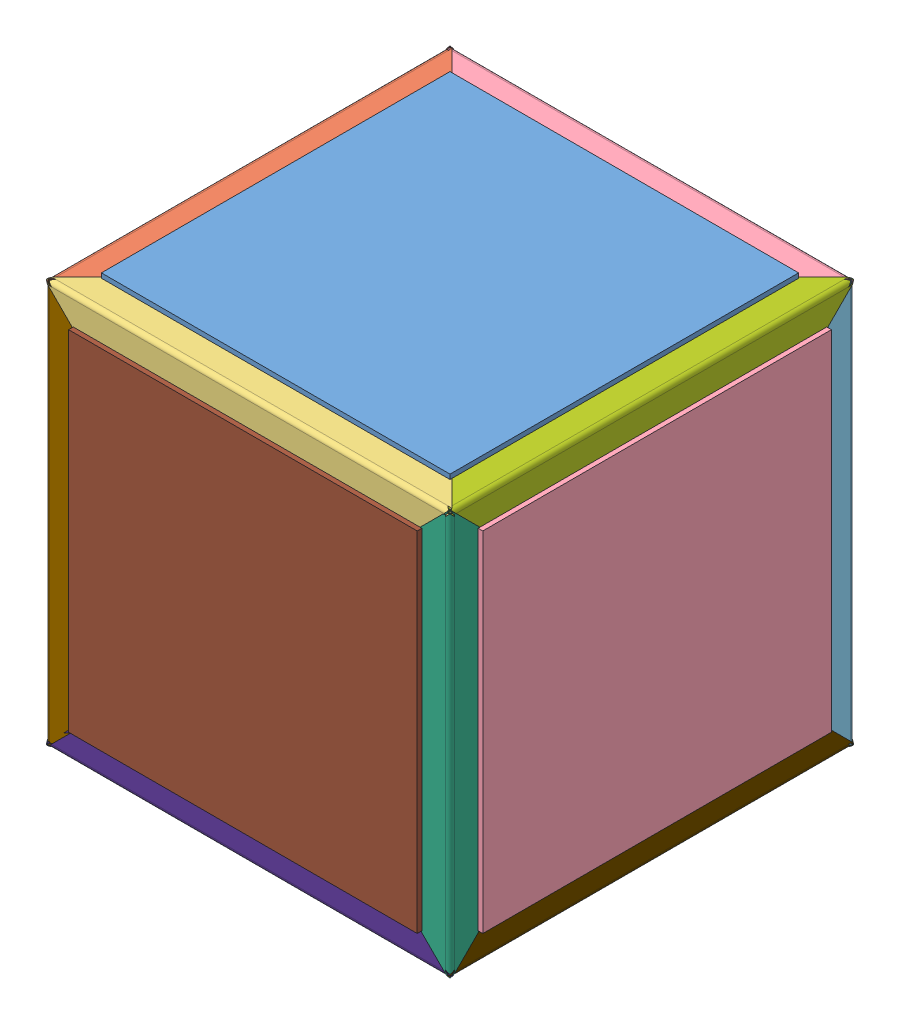
SolidWorks assembly cube_04, configuration cube04. Lengths in mm.
Overall size (140.33 140.33 140.33).
30 component instances, 30 part files, 92 mates.
Components (placement in the parent):
- pr^cube_04-28: pr^cube_04 [cube01] x (-1 0 0) z (0 0 1) (virtual)
- dr1^cube_04-55: dr1^cube_04 [cube01] at (-67.9746 68.58 0) x (0 -1 0) z (0 0 1) (virtual)
- dr2^cube_04-37: dr2^cube_04 [cube01] at (0 68.58 67.9746) x (0 -1 0) z (1 0 0) (virtual)
- dr3^cube_04-33: dr3^cube_04 [cube01] at (0 68.58 -67.9746) x (0 -1 0) z (-1 0 0) (virtual)
- br1^cube_04-49: br1^cube_04 [Default] at (0 43.18 -43.18) x (0 0 1) z (-1 0 0) (virtual)
- br2^cube_04-61: br2^cube_04 [Default] at (-43.18 43.18 0) (virtual)
- br3^cube_04-46: br3^cube_04 [Default] at (0 43.18 43.18) x (0 0 -1) z (1 0 0) (virtual)
- pg^cube_04-20: pg^cube_04 [cube01] x (0 -1 0) z (0 0 1) (virtual)
- dg1^cube_04-38: dg1^cube_04 [cube01] at (-68.58 0 67.9746) x (1 0 0) z (0 1 0) (virtual)
- dg2^cube_04-41: dg2^cube_04 [cube01] at (-68.58 -67.9746 0) (virtual)
- dg3^cube_04-34: dg3^cube_04 [cube01] at (-68.58 0 -67.9746) x (1 0 0) z (0 -1 0) (virtual)
- bg1^cube_04-47: bg1^cube_04 [Default] at (-43.18 -43.18 0) x (0 1 0) z (0 0 1) (virtual)
- bg2^cube_04-44: bg2^cube_04 [Default] at (-43.18 0 43.18) x (0 0 -1) z (0 1 0) (virtual)
- bg3^cube_04-40: bg3^cube_04 [Default] at (-43.18 0 -43.18) x (0 0 1) z (0 -1 0) (virtual)
- py^cube_04-21: py^cube_04 [cube01] at origin (virtual)
- dy1^cube_04-35: dy1^cube_04 [cube01] at (0 -68.58 -67.9746) x (0 1 0) z (1 0 0) (virtual)
- dy2^cube_04-39: dy2^cube_04 [cube01] at (0 -68.58 67.9746) x (0 1 0) z (-1 0 0) (virtual)
- dy3^cube_04-42: dy3^cube_04 [cube01] at (67.9746 -68.58 0) x (0 1 0) z (0 0 1) (virtual)
- by1^cube_04-41: by1^cube_04 [Default] at (0 -43.18 -43.18) x (0 0 1) z (1 0 0) (virtual)
- by2^cube_04-45: by2^cube_04 [Default] at (0 -43.18 43.18) x (0 0 -1) z (-1 0 0) (virtual)
- by3^cube_04-48: by3^cube_04 [Default] at (43.18 -43.18 0) x (-1 0 0) z (0 0 1) (virtual)
- po^cube_04-22: po^cube_04 [cube01] x (0 1 0) z (0 0 1) (virtual)
- do1^cube_04-36: do1^cube_04 [cube01] at (68.58 0 -67.9746) x (-1 0 0) z (0 1 0) (virtual)
- do2^cube_04-40: do2^cube_04 [cube01] at (68.58 0 67.9746) x (-1 0 0) z (0 -1 0) (virtual)
- do3^cube_04-47: do3^cube_04 [cube01] at (68.58 67.9746 0) x (-1 0 0) z (0 0 1) (virtual)
- bo1^cube_04-42: bo1^cube_04 [Default] at (43.18 0 -43.18) x (0 0 1) z (0 1 0) (virtual)
- bo2^cube_04-46: bo2^cube_04 [Default] at (43.18 0 43.18) x (0 0 -1) z (0 -1 0) (virtual)
- bo3^cube_04-62: bo3^cube_04 [Default] at (43.18 43.18 0) x (0 -1 0) z (0 0 1) (virtual)
- pc^cube_04-18: pc^cube_04 [cube01] x (-1 0 0) z (0 -1 0) (virtual)
- pb^cube_04-21: pb^cube_04 [cube01] x (-1 0 0) z (0 1 0) (virtual)
Mates (geometry in assembly coordinates):
- Coincident1: coincident anti-aligned: plane of pr^cube_04-28 through (59.055 68.58 -59.055) normal (0 -1 0); plane of br1^cube_04-49 through (-39.624 68.58 -43.18) normal (0 1 0)
- Coincident2: coincident anti-aligned: plane of pr^cube_04-28 through (59.055 68.58 -59.055) normal (0 -1 0); plane of br2^cube_04-61 through (-43.18 68.58 39.624) normal (0 1 0)
- Coincident3: coincident anti-aligned: plane of pr^cube_04-28 through (59.055 68.58 -59.055) normal (0 -1 0); plane of br3^cube_04-46 through (39.624 68.58 43.18) normal (0 1 0)
- Coincident4: coincident anti-aligned: plane of pr^cube_04-28 through (59.055 68.58 -59.055) normal (0 -1 0); plane of bo3^cube_04-62 through (43.18 68.58 39.624) normal (0 1 0)
- Coincident5: coincident anti-aligned: plane of pr^cube_04-28 through (59.055 68.58 -59.055) normal (0 -1 0); plane of dr3^cube_04-33 through (0 68.58 -136.5546) normal (0 1 0)
- Coincident6: coincident anti-aligned: plane of pr^cube_04-28 through (59.055 68.58 -59.055) normal (0 -1 0); plane of dr1^cube_04-55 through (-136.5546 68.58 0) normal (0 1 0)
- Coincident7: coincident anti-aligned: plane of pr^cube_04-28 through (59.055 68.58 -59.055) normal (0 -1 0); plane of do3^cube_04-47 through (-0.6054 68.58 0) normal (0 1 0)
- Coincident8: coincident anti-aligned: plane of pr^cube_04-28 through (59.055 68.58 -59.055) normal (0 -1 0); plane of dr2^cube_04-37 through (0 68.58 136.5546) normal (0 1 0)
- Coincident34: coincident anti-aligned: plane of pb^cube_04-21 through (59.055 -59.055 -68.58) normal (0 0 1); plane of by1^cube_04-41 through (39.624 -43.18 -68.58) normal (0 0 -1)
- Coincident35: coincident anti-aligned: plane of pb^cube_04-21 through (59.055 -59.055 -68.58) normal (0 0 1); plane of bo1^cube_04-42 through (43.18 39.624 -68.58) normal (0 0 -1)
- Coincident36: coincident anti-aligned: plane of pb^cube_04-21 through (59.055 -59.055 -68.58) normal (0 0 1); plane of br1^cube_04-49 through (-39.624 43.18 -68.58) normal (0 0 -1)
- Coincident37: coincident anti-aligned: plane of pb^cube_04-21 through (59.055 -59.055 -68.58) normal (0 0 1); plane of bg3^cube_04-40 through (-43.18 -39.624 -68.58) normal (0 0 -1)
- Coincident38: coincident anti-aligned: plane of pb^cube_04-21 through (59.055 -59.055 -68.58) normal (0 0 1); plane of dg3^cube_04-34 through (0.6054 0 -68.58) normal (0 0 -1)
- Coincident39: coincident anti-aligned: plane of pb^cube_04-21 through (59.055 -59.055 -68.58) normal (0 0 1); plane of dr3^cube_04-33 through (0 -0.6054 -68.58) normal (0 0 -1)
- Coincident40: coincident anti-aligned: plane of pb^cube_04-21 through (59.055 -59.055 -68.58) normal (0 0 1); plane of do1^cube_04-36 through (-0.6054 0 -68.58) normal (0 0 -1)
- Coincident41: coincident anti-aligned: plane of pb^cube_04-21 through (59.055 -59.055 -68.58) normal (0 0 1); plane of dy1^cube_04-35 through (0 0.6054 -68.58) normal (0 0 -1)
- Coincident42: coincident anti-aligned: plane of pc^cube_04-18 through (59.055 59.055 68.58) normal (0 0 -1); plane of bo2^cube_04-46 through (43.18 -39.624 68.58) normal (0 0 1)
- Coincident43: coincident anti-aligned: plane of pc^cube_04-18 through (59.055 59.055 68.58) normal (0 0 -1); plane of br3^cube_04-46 through (39.624 43.18 68.58) normal (0 0 1)
- Coincident44: coincident anti-aligned: plane of pc^cube_04-18 through (59.055 59.055 68.58) normal (0 0 -1); plane of bg2^cube_04-44 through (-43.18 39.624 68.58) normal (0 0 1)
- Coincident45: coincident anti-aligned: plane of pc^cube_04-18 through (59.055 59.055 68.58) normal (0 0 -1); plane of by2^cube_04-45 through (-39.624 -43.18 68.58) normal (0 0 1)
- Coincident46: coincident anti-aligned: plane of pc^cube_04-18 through (59.055 59.055 68.58) normal (0 0 -1); plane of do2^cube_04-40 through (-0.6054 0 68.58) normal (0 0 1)
- Coincident47: coincident anti-aligned: plane of pc^cube_04-18 through (59.055 59.055 68.58) normal (0 0 -1); plane of dy2^cube_04-39 through (0 0.6054 68.58) normal (0 0 1)
- Coincident48: coincident anti-aligned: plane of pc^cube_04-18 through (59.055 59.055 68.58) normal (0 0 -1); plane of dg1^cube_04-38 through (0.6054 0 68.58) normal (0 0 1)
- Coincident49: coincident anti-aligned: plane of pc^cube_04-18 through (59.055 59.055 68.58) normal (0 0 -1); plane of dr2^cube_04-37 through (0 -0.6054 68.58) normal (0 0 1)
- Coincident50: coincident anti-aligned: plane of pg^cube_04-20 through (-68.58 59.055 -59.055) normal (1 0 0); plane of bg3^cube_04-40 through (-68.58 -39.624 -43.18) normal (-1 0 0)
- Coincident51: coincident anti-aligned: plane of pg^cube_04-20 through (-68.58 59.055 -59.055) normal (1 0 0); plane of bg1^cube_04-47 through (-68.58 -43.18 39.624) normal (-1 0 0)
- Coincident52: coincident anti-aligned: plane of pg^cube_04-20 through (-68.58 59.055 -59.055) normal (1 0 0); plane of bg2^cube_04-44 through (-68.58 39.624 43.18) normal (-1 0 0)
- Coincident53: coincident anti-aligned: plane of pg^cube_04-20 through (-68.58 59.055 -59.055) normal (1 0 0); plane of dr1^cube_04-55 through (-68.58 -0.6054 0) normal (-1 0 0)
- Coincident54: coincident anti-aligned: plane of pg^cube_04-20 through (-68.58 59.055 -59.055) normal (1 0 0); plane of dg3^cube_04-34 through (-68.58 0 -136.5546) normal (-1 0 0)
- Coincident55: coincident anti-aligned: plane of pg^cube_04-20 through (-68.58 59.055 -59.055) normal (1 0 0); plane of dg2^cube_04-41 through (-68.58 -136.5546 0) normal (-1 0 0)
- Coincident56: coincident anti-aligned: plane of pg^cube_04-20 through (-68.58 59.055 -59.055) normal (1 0 0); plane of dg1^cube_04-38 through (-68.58 0 136.5546) normal (-1 0 0)
- Coincident99: coincident anti-aligned: plane of pg^cube_04-20 through (-68.58 59.055 -59.055) normal (1 0 0); plane of br2^cube_04-61 through (-68.58 43.18 39.624) normal (-1 0 0)
- Coincident57: coincident anti-aligned: plane of py^cube_04-21 through (-59.055 -68.58 -59.055) normal (0 1 0); plane of by3^cube_04-48 through (43.18 -68.58 39.624) normal (0 -1 0)
- Coincident58: coincident anti-aligned: plane of py^cube_04-21 through (-59.055 -68.58 -59.055) normal (0 1 0); plane of by2^cube_04-45 through (-39.624 -68.58 43.18) normal (0 -1 0)
- Coincident59: coincident anti-aligned: plane of py^cube_04-21 through (-59.055 -68.58 -59.055) normal (0 1 0); plane of bg1^cube_04-47 through (-43.18 -68.58 39.624) normal (0 -1 0)
- Coincident60: coincident anti-aligned: plane of py^cube_04-21 through (-59.055 -68.58 -59.055) normal (0 1 0); plane of by1^cube_04-41 through (39.624 -68.58 -43.18) normal (0 -1 0)
- Coincident61: coincident anti-aligned: plane of py^cube_04-21 through (-59.055 -68.58 -59.055) normal (0 1 0); plane of dy3^cube_04-42 through (136.5546 -68.58 0) normal (0 -1 0)
- Coincident62: coincident anti-aligned: plane of py^cube_04-21 through (-59.055 -68.58 -59.055) normal (0 1 0); plane of dy2^cube_04-39 through (0 -68.58 136.5546) normal (0 -1 0)
- Coincident63: coincident anti-aligned: plane of py^cube_04-21 through (-59.055 -68.58 -59.055) normal (0 1 0); plane of dg2^cube_04-41 through (0.6054 -68.58 0) normal (0 -1 0)
- Coincident64: coincident anti-aligned: plane of py^cube_04-21 through (-59.055 -68.58 -59.055) normal (0 1 0); plane of dy1^cube_04-35 through (0 -68.58 -136.5546) normal (0 -1 0)
- Coincident65: coincident anti-aligned: plane of po^cube_04-22 through (68.58 -59.055 -59.055) normal (-1 0 0); plane of bo1^cube_04-42 through (68.58 39.624 -43.18) normal (1 0 0)
- Coincident66: coincident anti-aligned: plane of po^cube_04-22 through (68.58 -59.055 -59.055) normal (-1 0 0); plane of by3^cube_04-48 through (68.58 -43.18 39.624) normal (1 0 0)
- Coincident67: coincident anti-aligned: plane of po^cube_04-22 through (68.58 -59.055 -59.055) normal (-1 0 0); plane of bo2^cube_04-46 through (68.58 -39.624 43.18) normal (1 0 0)
- Coincident68: coincident anti-aligned: plane of po^cube_04-22 through (68.58 -59.055 -59.055) normal (-1 0 0); plane of bo3^cube_04-62 through (68.58 43.18 39.624) normal (1 0 0)
- Coincident69: coincident anti-aligned: plane of po^cube_04-22 through (68.58 -59.055 -59.055) normal (-1 0 0); plane of do2^cube_04-40 through (68.58 0 136.5546) normal (1 0 0)
- Coincident70: coincident anti-aligned: plane of po^cube_04-22 through (68.58 -59.055 -59.055) normal (-1 0 0); plane of do3^cube_04-47 through (68.58 136.5546 0) normal (1 0 0)
- Coincident71: coincident anti-aligned: plane of po^cube_04-22 through (68.58 -59.055 -59.055) normal (-1 0 0); plane of do1^cube_04-36 through (68.58 0 -136.5546) normal (1 0 0)
- Coincident72: coincident anti-aligned: plane of po^cube_04-22 through (68.58 -59.055 -59.055) normal (-1 0 0); plane of dy3^cube_04-42 through (68.58 0.6054 0) normal (1 0 0)
- Coincident73: coincident aligned: plane of assembly through (0 0 0) normal (0 0 1); plane of dy3^cube_04-42 through (67.9746 -68.58 0) normal (0 0 1)
- Coincident74: coincident aligned: plane of assembly through (0 0 0) normal (0 0 1); plane of by3^cube_04-48 through (43.18 -43.18 0) normal (0 0 1)
- Coincident75: coincident aligned: plane of assembly through (0 0 0) normal (0 0 1); plane of bo3^cube_04-62 through (43.18 43.18 0) normal (0 0 1)
- Coincident76: coincident aligned: plane of assembly through (0 0 0) normal (0 0 1); plane of do3^cube_04-47 through (68.58 67.9746 0) normal (0 0 1)
- Coincident77: coincident aligned: plane of assembly through (0 0 0) normal (0 0 1); plane of dg2^cube_04-41 through (-68.58 -67.9746 0) normal (0 0 1)
- Coincident78: coincident aligned: plane of assembly through (0 0 0) normal (0 0 1); plane of bg1^cube_04-47 through (-43.18 -43.18 0) normal (0 0 1)
- Coincident79: coincident aligned: plane of assembly through (0 0 0) normal (0 0 1); plane of dr1^cube_04-55 through (-67.9746 68.58 0) normal (0 0 1)
- Coincident80: coincident aligned: plane of assembly through (0 0 0) normal (0 0 1); plane of br2^cube_04-61 through (-43.18 43.18 0) normal (0 0 1)
- Coincident81: coincident aligned: plane of assembly through (0 0 0) normal (0 1 0); plane of bo1^cube_04-42 through (43.18 0 -43.18) normal (0 1 0)
- Coincident82: coincident aligned: plane of assembly through (0 0 0) normal (0 1 0); plane of py^cube_04-21 through (0 0 0) normal (0 1 0)
- Coincident83: coincident aligned: plane of assembly through (0 0 0) normal (0 1 0); plane of do1^cube_04-36 through (68.58 0 -67.9746) normal (0 1 0)
- Coincident84: coincident anti-aligned: plane of assembly through (0 0 0) normal (0 1 0); plane of bg3^cube_04-40 through (-43.18 0 -43.18) normal (0 -1 0)
- Coincident85: coincident anti-aligned: plane of assembly through (0 0 0) normal (0 1 0); plane of dg3^cube_04-34 through (-68.58 0 -67.9746) normal (0 -1 0)
- Coincident86: coincident aligned: plane of assembly through (0 0 0) normal (0 1 0); plane of dg1^cube_04-38 through (-68.58 0 67.9746) normal (0 1 0)
- Coincident87: coincident aligned: plane of assembly through (0 0 0) normal (0 1 0); plane of bg2^cube_04-44 through (-43.18 0 43.18) normal (0 1 0)
- Coincident88: coincident anti-aligned: plane of assembly through (0 0 0) normal (0 1 0); plane of bo2^cube_04-46 through (43.18 0 43.18) normal (0 -1 0)
- Coincident89: coincident anti-aligned: plane of assembly through (0 0 0) normal (0 1 0); plane of do2^cube_04-40 through (68.58 0 67.9746) normal (0 -1 0)
- Coincident90: coincident anti-aligned: plane of assembly through (0 0 0) normal (1 0 0); plane of by2^cube_04-45 through (0 -43.18 43.18) normal (-1 0 0)
- Coincident91: coincident anti-aligned: plane of assembly through (0 0 0) normal (1 0 0); plane of dy2^cube_04-39 through (0 -68.58 67.9746) normal (-1 0 0)
- Coincident92: coincident aligned: plane of assembly through (0 0 0) normal (1 0 0); plane of pg^cube_04-20
- Coincident93: coincident aligned: plane of assembly through (0 0 0) normal (1 0 0); plane of dr2^cube_04-37 through (0 68.58 67.9746) normal (1 0 0)
- Coincident94: coincident aligned: plane of assembly through (0 0 0) normal (1 0 0); plane of br3^cube_04-46 through (0 43.18 43.18) normal (1 0 0)
- Coincident95: coincident anti-aligned: plane of assembly through (0 0 0) normal (1 0 0); plane of dr3^cube_04-33 through (0 68.58 -67.9746) normal (-1 0 0)
- Coincident96: coincident anti-aligned: plane of assembly through (0 0 0) normal (1 0 0); plane of br1^cube_04-49 through (0 43.18 -43.18) normal (-1 0 0)
- Coincident97: coincident aligned: plane of assembly through (0 0 0) normal (1 0 0); plane of by1^cube_04-41 through (0 -43.18 -43.18) normal (1 0 0)
- Coincident98: coincident aligned: plane of assembly through (0 0 0) normal (1 0 0); plane of dy1^cube_04-35 through (0 -68.58 -67.9746) normal (1 0 0)
- Coincident100: coincident anti-aligned: plane of pr^cube_04-28; plane of assembly through (0 0 0) normal (1 0 0)
- Coincident101: coincident aligned: plane of pr^cube_04-28 through (0 0 0) normal (0 0 1); plane of assembly through (0 0 0) normal (0 0 1)
- Coincident102: coincident anti-aligned: plane of pr^cube_04-28; plane of assembly through (0 0 0) normal (0 1 0)
- Coincident106: coincident anti-aligned: plane of pg^cube_04-20; plane of assembly through (0 0 0) normal (0 1 0)
- Coincident107: coincident aligned: plane of pg^cube_04-20; plane of assembly through (0 0 0) normal (1 0 0)
- Coincident108: coincident aligned: plane of pg^cube_04-20 through (0 0 0) normal (0 0 1); plane of assembly through (0 0 0) normal (0 0 1)
- Coincident109: coincident aligned: plane of py^cube_04-21 through (0 0 0) normal (0 0 1); plane of assembly through (0 0 0) normal (0 0 1)
- Coincident110: coincident aligned: plane of py^cube_04-21 through (0 0 0) normal (0 1 0); plane of assembly through (0 0 0) normal (0 1 0)
- Coincident111: coincident aligned: plane of py^cube_04-21 through (0 0 0) normal (1 0 0); plane of assembly through (0 0 0) normal (1 0 0)
- Coincident112: coincident aligned: plane of po^cube_04-22 through (0 0 0) normal (0 0 1); plane of assembly through (0 0 0) normal (0 0 1)
- Coincident113: coincident anti-aligned: plane of po^cube_04-22; plane of assembly through (0 0 0) normal (1 0 0)
- Coincident114: coincident aligned: plane of po^cube_04-22; plane of assembly through (0 0 0) normal (0 1 0)
- Coincident115: coincident anti-aligned: plane of pc^cube_04-18 through (0 0 0) normal (0 -1 0); plane of assembly through (0 0 0) normal (0 1 0)
- Coincident116: coincident anti-aligned: plane of pc^cube_04-18; plane of assembly through (0 0 0) normal (0 0 1)
- Coincident117: coincident anti-aligned: plane of pc^cube_04-18; plane of assembly through (0 0 0) normal (1 0 0)
- Coincident118: coincident aligned: plane of pb^cube_04-21 through (0 0 0) normal (0 1 0); plane of assembly through (0 0 0) normal (0 1 0)
- Coincident119: coincident aligned: plane of pb^cube_04-21; plane of assembly through (0 0 0) normal (0 0 1)
- Coincident120: coincident anti-aligned: line of pb^cube_04-21 through (0.8731 -0.8731 0) axis (0 0 -1); plane of assembly through (0 0 0) normal (1 0 0)
